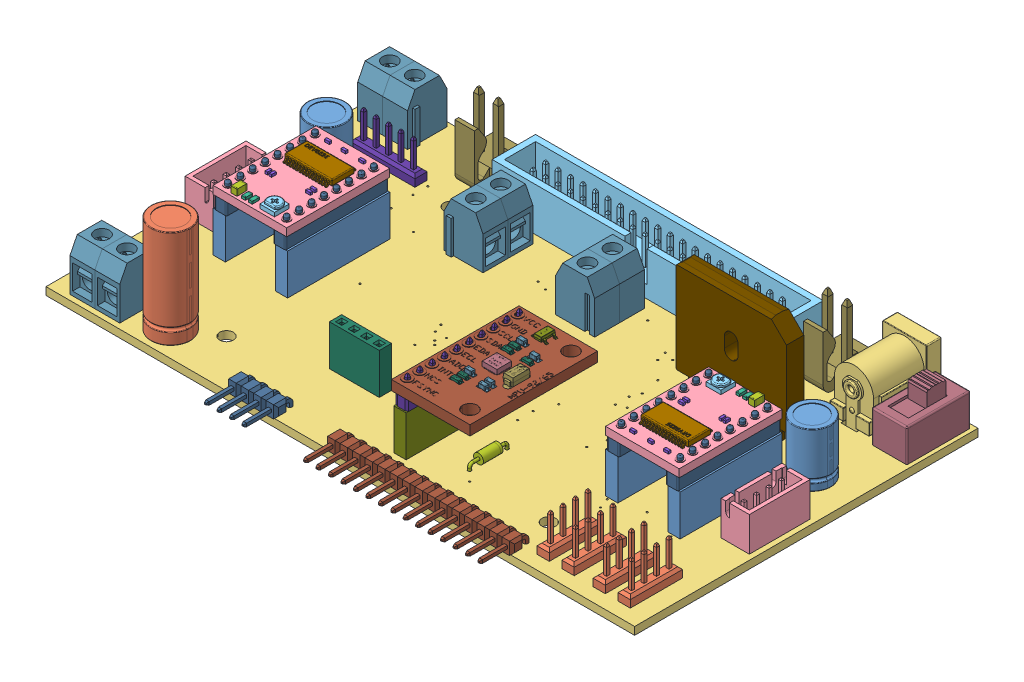
SolidWorks assembly RILey_PCB_V2, configuration Default. Lengths in mm.
Overall size (120 36.8 77.07).
114 component instances, 35 part files, 11 mates.
Components (placement in the parent):
- RILey-PCB_V2.0.step-1: RILey-PCB_V2.0.step [Default] at (-30.3949 55.9091 134.4073) x (1 0 0) z (0 1 0) size (120 77.07 36.8)
  - Packages.step-1: Packages.step [Default] at origin size (117.53 77.07 36.8)
    - CAPPRD250W50D655H1250.step-1: CAPPRD250W50D655H1250.step [Default] at (10.16 48.26 1.57) x (-1 0 0) z (0 0 1) size (7.62 7.6 12.92)
      - Model.step-1: Model.step [Default] at (1.2482 -0.0007 0.1237) size (7.62 7.6 12.92)
    - CAPPRD250W50D655H1250_1.step-1: CAPPRD250W50D655H1250_1.step [Default] at (110.49 44.45 1.57) size (7.62 7.6 12.92)
      - Model.step-1: Model.step [Default] at (1.2482 -0.0007 0.1237) size (7.62 7.6 12.92)
    - ELECTROLYTIC_CAPACITOR.step-1: ELECTROLYTIC_CAPACITOR.step [Default] at (20.32 5.08 1.57) size (8.02 8 21.92)
      - Model (1).step-1: Model (1).step [Default] at origin size (8.02 8 21.92)
    - 733980-62.step-1: 733980-62.step [Default] at (106.68 66.04 1.57) x (-1 0 0) z (0 0 1) size (9.55 14.2 15)
      - DS-210 v1.step-1: DS-210 v1.step [Default] at (-0.0014 -5.2814 0) x (-1 0 0) z (0 0 1) size (9.55 14.2 15)
    - B4B-XH-A_LF__SN_.step-1: B4B-XH-A_LF__SN_.step [Default] at (5.08 29.21 1.57) x (0 1 0) z (0 0 1) size (12.4 5.75 10.45)
      - JST XH 4 B4B-XH-A v1.step-1: JST XH 4 B4B-XH-A v1.step [Default] at (3.6633 0.5127 0.0202) x (1 0 0) z (0 -1 0) size (12.4 10.45 5.75)
    - B4B-XH-A_LF__SN_.step-2: B4B-XH-A_LF__SN_.step [Default] at (115.57 34.29 1.57) x (0 -1 0) z (0 0 1) size (12.4 5.75 10.45)
      - JST XH 4 B4B-XH-A v1.step-1: JST XH 4 B4B-XH-A v1.step [Default] at (3.6633 0.5127 0.0202) x (1 0 0) z (0 -1 0) size (12.4 10.45 5.75)
    - MC-254-40-00-ST-DIP.step-1: MC-254-40-00-ST-DIP.step [Default] at (61.214 63.5 1.57) size (58.67 8.85 11.85)
      - MC-254-40-00-ST-DIP v1.step-1: MC-254-40-00-ST-DIP v1.step [Default] at (-24.13 -1.27 0) size (58.67 8.85 11.85)
        - Model (2).step-1: Model (2).step [Default] at (0 2.54 0) size (58.67 8.85 11.85)
    - TSOP6_SOT457.step-1: TSOP6_SOT457.step [Default] at (17.78 48.26 0) x (-1 0 0) z (0 0 -1) size (3 3.1 1.1)
      - Model (3).step-1: Model (3).step [Default] at origin size (3 3.1 1.1)
    - ZENER-TH.step-1: ZENER-TH.step [Default] at (75.565 14.605 1.57) x (0 1 0) z (0 0 1) size (8.22 2 4.02)
      - Model (4).step-1: Model (4).step [Default] x (-1 0 0) z (0 0 1) size (8.22 2 4.02)
    - 1812L300MR.step-1: 1812L300MR.step [Default] at (71.0315 17.78 0) x (0 -1 0) z (0 0 -1) size (4.73 3.41 1)
      - Model (5).step-1: Model (5).step [Default] at origin size (4.73 3.41 1)
    - 2920L400_15MR.step-1: 2920L400_15MR.step [Default] at (109.22 52.07 0) x (1 0 0) z (0 0 -1) size (7.98 5.44 1.6)
      - Model (6).step-1: Model (6).step [Default] at origin size (7.98 5.44 1.6)
    - MA04-1W.step-1: MA04-1W.step [Default] at (42.0116 3.8608 1.57) x (-1 0 0) z (0 0 1) size (10.16 9.88 5.54)
      - Model (7).step-1: Model (7).step [Default] at (3.81 -0.002 0) x (-1 0 0) z (0 0 1) size (10.16 9.89 5.54)
    - MA15-1W.step-1: MA15-1W.step [Default] at (76.2 3.81 1.57) x (-1 0 0) z (0 0 1) size (38.1 9.89 5.54)
      - Model (8).step-1: Model (8).step [Default] at (17.78 0 0) x (-1 0 0) z (0 0 1) size (38.1 9.89 5.54)
    - KK41791-4020_2-PIN.step-1: KK41791-4020_2-PIN.step [Default] at (96.52 64.77 1.57) x (-1 0 0) z (0 0 1) size (7.77 10.01 17.02)
      - Molex-kk-396 v2.step-1: Molex-kk-396 v2.step [Default] at (0.0973 -2.0339 0.4801) x (1 0 0) z (0 -1 0) size (7.77 17.02 10.01)
        - 1.step-1: 1.step [Default] at (-0.1266 1.3496 -0.3443) size (7.77 17.02 10.01)
    - KK41791-4020_2-PIN_1.step-1: KK41791-4020_2-PIN_1.step [Default] at (25.4 64.77 1.57) x (-1 0 0) z (0 0 1) size (7.77 10.01 17.02)
      - Molex-kk-396 v2_1.step-1: Molex-kk-396 v2_1.step [Default] at (0.0973 -2.0339 0.4801) x (1 0 0) z (0 -1 0) size (7.77 17.02 10.01)
        - 1.step-1: 1.step [Default] at (-0.1266 1.3496 -0.3443) size (7.77 17.02 10.01)
    - 1000-SERIES(SPDT).step-1: 1000-SERIES(SPDT).step [Default] at (115.6208 62.7634 1.57) size (7.2 13 13.1)
      - SS-12M11G3 v2.step-1: SS-12M11G3 v2.step [Default] at origin size (7.2 13 13.1)
    - W237-102.step-1: W237-102.step [Default] at (7.5692 66.3194 1.57) size (10.66 8 14)
      - Schraubklemme_Blau_300V_16A_2P v1.step-1: Schraubklemme_Blau_300V_16A_2P v1.step [Default] at (-0.2451 0.529 2.8414) x (0 1 0) z (0 0 1) size (8 10.66 14)
        - Schraubklemme_Blau_300V_16A.step-1: Schraubklemme_Blau_300V_16A.step [Default] at (2.2082 -5.3326 -3) size (8 5.58 14)
        - Schraubklemme_Blau_300V_16A.step-2: Schraubklemme_Blau_300V_16A.step [Default] at (2.2082 -0.2526 -3) size (8 5.58 14)
    - W237-102_1.step-1: W237-102_1.step [Default] at (8.89 3.81 1.57) x (-1 0 0) z (0 0 1) size (10.66 8 14)
      - Schraubklemme_Blau_300V_16A_2P v1_1.step-1: Schraubklemme_Blau_300V_16A_2P v1_1.step [Default] at (-0.2451 0.529 2.8414) x (0 1 0) z (0 0 1) size (8 10.66 14)
        - Schraubklemme_Blau_300V_16A.step-1: Schraubklemme_Blau_300V_16A.step [Default] at (2.2082 -5.3326 -3) size (8 5.58 14)
        - Schraubklemme_Blau_300V_16A.step-2: Schraubklemme_Blau_300V_16A.step [Default] at (2.2082 -0.2526 -3) size (8 5.58 14)
    - W237-102_2.step-1: W237-102_2.step [Default] at (59.5884 52.07 1.57) x (0 1 0) z (0 0 1) size (10.66 8 14)
      - Schraubklemme_Blau_300V_16A_2P v1_2.step-1: Schraubklemme_Blau_300V_16A_2P v1_2.step [Default] at (-0.2451 0.529 2.8414) x (0 1 0) z (0 0 1) size (8 10.66 14)
        - Schraubklemme_Blau_300V_16A.step-1: Schraubklemme_Blau_300V_16A.step [Default] at (2.2082 -5.3326 -3) size (8 5.58 14)
        - Schraubklemme_Blau_300V_16A.step-2: Schraubklemme_Blau_300V_16A.step [Default] at (2.2082 -0.2526 -3) size (8 5.58 14)
    - W237-102_3.step-1: W237-102_3.step [Default] at (39.37 52.07 1.57) x (0 -1 0) z (0 0 1) size (10.66 8 14)
      - Schraubklemme_Blau_300V_16A_2P v1_3.step-1: Schraubklemme_Blau_300V_16A_2P v1_3.step [Default] at (-0.2451 0.529 2.8414) x (0 1 0) z (0 0 1) size (8 10.66 14)
        - Schraubklemme_Blau_300V_16A.step-1: Schraubklemme_Blau_300V_16A.step [Default] at (2.2082 -5.3326 -3) size (8 5.58 14)
        - Schraubklemme_Blau_300V_16A.step-2: Schraubklemme_Blau_300V_16A.step [Default] at (2.2082 -0.2526 -3) size (8 5.58 14)
    - FE04-1.step-1: FE04-1.step [Default] at (52.2732 15.6464 1.57) x (-1 0 0) z (0 0 1) size (10.16 2.5 11.3)
    - FE10-1.step-1: FE10-1.step [Default] at (66.04 19.0691 1.57) x (0 -1 0) z (0 0 1) size (25.9 2.5 11.3)
    - MA05-1_S.step-1: MA05-1_S.step [Default] at (13.97 55.88 1.57) x (-1 0 0) z (0 0 1) size (13.2 2.5 11)
    - DIODE-BRIDGE.step-1: DIODE-BRIDGE.step [Default] at (92.71 48.26 1.57) size (22.51 3.56 36.8)
    - FE08-1.step-1: FE08-1.step [Default] at (25.4 33.02 1.57) x (0 1 0) z (0 0 1) size (20.82 2.5 11.3)
    - FE08-1.step-2: FE08-1.step [Default] at (12.7 33.02 1.57) x (0 1 0) z (0 0 1) size (20.82 2.5 11.3)
    - FE08-1.step-3: FE08-1.step [Default] at (95.25 30.48 1.57) x (0 -1 0) z (0 0 1) size (20.82 2.5 11.3)
    - FE08-1.step-4: FE08-1.step [Default] at (107.95 30.48 1.57) x (0 -1 0) z (0 0 1) size (20.82 2.5 11.3)
    - MA04-1_S.step-1: MA04-1_S.step [Default] at (99.06 7.62 1.57) x (0 -1 0) z (0 0 1) size (10.66 2.5 11)
    - MA04-1_S.step-2: MA04-1_S.step [Default] at (104.14 7.62 1.57) x (0 -1 0) z (0 0 1) size (10.66 2.5 11)
    - MA04-1_S.step-3: MA04-1_S.step [Default] at (110.49 7.62 1.57) x (0 -1 0) z (0 0 1) size (10.66 2.5 11)
    - MA04-1_S.step-4: MA04-1_S.step [Default] at (115.57 7.62 1.57) x (0 -1 0) z (0 0 1) size (10.66 2.5 11)
  - Board.step-1: Board.step [Default] at origin size (120 70 1.57)
- DRV 8825 With Headers Assem-1: DRV 8825 With Headers Assem [Default] at (-1.0467 51.8574 109.5035) x (0 0 -1) z (0 1 0) size (21 15 10.9)
  - PCB-1: PCB [Default] at (8.1162 10.2982 16.4218) size (21 15 1.8)
  - SMD Pot-1: SMD Pot [Default] at (-0.2134 7.4613 18.0218) x (0 -1 0) z (0 0 1) size (3 3 1.3)
  - 0603 Resistor-1: 0603 Resistor [Default] at (-1.0068 10.8561 18.0218) size (1.5 0.8 0.5)
  - 0603 Resistor-2: 0603 Resistor [Default] at (-1.0286 12.2306 18.0218) size (1.5 0.8 0.5)
  - 0805 Capacitor-1: 0805 Capacitor [Default] at (-0.8941 14.0417 18.0218) size (2 1.25 1.25)
  - 0402 Resistor-1: 0402 Resistor [Default] at (16.8896 6.6863 18.0218) x (0 -1 0) z (0 0 1) size (1 0.68 0.66)
  - 0402 Resistor-2: 0402 Resistor [Default] at (16.8896 10.308 18.0218) x (0 -1 0) z (0 0 1) size (1 0.68 0.66)
  - 0402 Resistor-3: 0402 Resistor [Default] at (16.8896 13.6408 18.0218) x (0 -1 0) z (0 0 1) size (1 0.68 0.66)
  - 0402 Resistor-4: 0402 Resistor [Default] at (6.8882 6.5987 18.0218) x (0 -1 0) z (0 0 1) size (1 0.68 0.66)
  - 0402 Resistor-5: 0402 Resistor [Default] at (5.9719 6.5987 18.0218) x (0 -1 0) z (0 0 1) size (1 0.68 0.66)
  - 0402 Resistor-6: 0402 Resistor [Default] at (5.456 14.3274 18.0218) size (1 0.68 0.66)
  - 0402 Resistor-7: 0402 Resistor [Default] at (5.456 13.4855 18.0218) size (1 0.68 0.66)
  - DRV8825 IC-1: DRV8825 IC [Default] at (11.7347 10.2312 18.0218) x (0 -1 0) z (0 0 1) size (9.6 6.2 1.2)
  - 8 pin Header-1: 8 pin Header [Default] at (8.1162 16.2982 13.9218) size (21 2.5 10.5)
  - 8 pin Header-2: 8 pin Header [Default] at (8.1162 4.2982 13.9218) size (21 2.5 10.5)
- DRV 8825 With Headers Assem-2: DRV 8825 With Headers Assem [Default] at (60.9069 51.8574 95.811) x (0 0 1) z (0 1 0) size (21 15 10.9)
  - PCB-1: PCB [Default] at (8.1162 10.2982 16.4218) size (21 15 1.8)
  - SMD Pot-1: SMD Pot [Default] at (-0.2134 7.4613 18.0218) x (0 -1 0) z (0 0 1) size (3 3 1.3)
  - 0603 Resistor-1: 0603 Resistor [Default] at (-1.0068 10.8561 18.0218) size (1.5 0.8 0.5)
  - 0603 Resistor-2: 0603 Resistor [Default] at (-1.0286 12.2306 18.0218) size (1.5 0.8 0.5)
  - 0805 Capacitor-1: 0805 Capacitor [Default] at (-0.8941 14.0417 18.0218) size (2 1.25 1.25)
  - 0402 Resistor-1: 0402 Resistor [Default] at (16.8896 6.6863 18.0218) x (0 -1 0) z (0 0 1) size (1 0.68 0.66)
  - 0402 Resistor-2: 0402 Resistor [Default] at (16.8896 10.308 18.0218) x (0 -1 0) z (0 0 1) size (1 0.68 0.66)
  - 0402 Resistor-3: 0402 Resistor [Default] at (16.8896 13.6408 18.0218) x (0 -1 0) z (0 0 1) size (1 0.68 0.66)
  - 0402 Resistor-4: 0402 Resistor [Default] at (6.8882 6.5987 18.0218) x (0 -1 0) z (0 0 1) size (1 0.68 0.66)
  - 0402 Resistor-5: 0402 Resistor [Default] at (5.9719 6.5987 18.0218) x (0 -1 0) z (0 0 1) size (1 0.68 0.66)
  - 0402 Resistor-6: 0402 Resistor [Default] at (5.456 14.3274 18.0218) size (1 0.68 0.66)
  - 0402 Resistor-7: 0402 Resistor [Default] at (5.456 13.4855 18.0218) size (1 0.68 0.66)
  - DRV8825 IC-1: DRV8825 IC [Default] at (11.7347 10.2312 18.0218) x (0 -1 0) z (0 0 1) size (9.6 6.2 1.2)
  - 8 pin Header-1: 8 pin Header [Default] at (8.1162 16.2982 13.9218) size (21 2.5 10.5)
  - 8 pin Header-2: 8 pin Header [Default] at (8.1162 4.2982 13.9218) size (21 2.5 10.5)
- MPU9250.STEP-1: MPU9250.STEP [Default] at (68.1451 69.3424 118.518) x (0 0 1) z (-1 0 0) size (26 3.91 16)
  - PCB.STEP-1: PCB.STEP [Default] at (-2.9998 1.0768 26) size (26 2.2 16)
  - C2.STEP-1: C2.STEP [Default] at (-2.4989 2.0768 21) x (0 0 -1) z (1 0 0) size (2 1.81 5.01)
  - MP92.STEP-1: MP92.STEP [Default] at (-2.9998 1.0968 25.5) x (0 0 -1) z (1 0 0) size (3.29 1.01 3.29)
  - C1_Predeterminado_Como mecanizada_.STEP-1: C1_Predeterminado_Como mecanizada_.STEP [Default] at (2.1384 1.0968 23.0905) x (0 0 1) z (-1 0 0) size (2.2 0.83 0.9)
  - C1_Predeterminado_Como mecanizada_.STEP-2: C1_Predeterminado_Como mecanizada_.STEP [Default] at (0.9102 1.0968 27.1044) x (0 0 1) z (-1 0 0) size (2.2 0.83 0.9)
  - C1_Predeterminado_Como mecanizada_.STEP-3: C1_Predeterminado_Como mecanizada_.STEP [Default] at (0.9102 1.0968 23.0905) x (0 0 1) z (-1 0 0) size (2.2 0.83 0.9)
  - C1_Predeterminado_Como mecanizada_.STEP-4: C1_Predeterminado_Como mecanizada_.STEP [Default] at (-8.3098 1.0968 23.0905) x (0 0 1) z (-1 0 0) size (2.2 0.83 0.9)
  - C1_Predeterminado_Como mecanizada_.STEP-5: C1_Predeterminado_Como mecanizada_.STEP [Default] at (-9.7098 1.0968 27.1044) x (0 0 1) z (-1 0 0) size (2.2 0.83 0.9)
  - R1.STEP-1: R1.STEP [Default] at (3.5484 1.1168 27.2144) x (0 0 -1) z (1 0 0) size (2.2 0.47 0.9)
  - R1.STEP-2: R1.STEP [Default] at (2.1484 1.1168 27.2144) x (0 0 -1) z (1 0 0) size (2.2 0.47 0.9)
  - R1.STEP-3: R1.STEP [Default] at (-6.8998 1.1168 23.2005) x (0 0 -1) z (1 0 0) size (2.2 0.47 0.9)
  - R1.STEP-4: R1.STEP [Default] at (-8.2998 1.1168 27.2144) x (0 0 -1) z (1 0 0) size (2.2 0.47 0.9)
  - R1.STEP-5: R1.STEP [Default] at (-6.8998 1.1168 27.2144) x (0 0 -1) z (1 0 0) size (2.2 0.47 0.9)
  - V1.STEP-1: V1.STEP [Default] at (-13.0785 1.5868 25.9) size (2.9 0.96 3.2)
- PinHeader10row-1: PinHeader10row [Default] at (36.9151 68.3191 125.4982) x (0 0 1) z (1 0 0) size (25.4 11.54 2.54)
Mates (geometry in assembly coordinates):
- ProfileCenter1: profile center = 1.85 mm anti-aligned: plane of PinHeader10row-1 through (36.9151 59.7791 125.4982) normal (0 -1 0); plane of RILey-PCB_V2.0.step-1/Packages.step-1/FE10-1.step-1 through (35.6451 61.6291 126.7682) normal (0 1 0)
- Concentric1: concentric: cylinder of RILey-PCB_V2.0.step-1/Board.step-1 through (35.6451 -144.0909 126.7682) axis (0 1 0) radius 0.5776; cylinder of MPU9250.STEP-1/PCB.STEP-1 through (35.6451 68.4191 126.7682) axis (0 1 0) radius 0.5
- Parallel3: parallel: plane of RILey-PCB_V2.0.step-1/Packages.step-1/FE10-1.step-1 through (34.3951 61.6291 115.3382) normal (-1 0 0); plane of MPU9250.STEP-1/PCB.STEP-1 through (34.1451 68.4191 115.5182) normal (-1 0 0)
- Parallel4: parallel: plane of RILey-PCB_V2.0.step-1/Packages.step-1/FE10-1.step-1 through (35.6451 61.6291 128.2882) normal (0 0 1); plane of MPU9250.STEP-1/PCB.STEP-1 through (42.1451 68.4191 128.5182) normal (0 0 1)
- Coincident3: coincident anti-aligned: plane of MPU9250.STEP-1/PCB.STEP-1 through (42.1451 68.3191 115.5182) normal (0 -1 0); plane of PinHeader10row-1 through (36.9151 68.3191 125.4982) normal (0 1 0)
- Width1: width: plane of DRV 8825 With Headers Assem-1/PCB-1 through (-3.8449 69.8791 111.8873) normal (1 0 0); plane of DRV 8825 With Headers Assem-1/PCB-1 through (-18.8449 69.8791 111.8873) normal (-1 0 0); plane of RILey-PCB_V2.0.step-1/Packages.step-1/FE08-1.step-2 through (-18.9449 61.6291 101.3873) normal (-1 0 0); plane of RILey-PCB_V2.0.step-1/Packages.step-1/FE08-1.step-1 through (-3.7449 61.6291 101.3873) normal (1 0 0)
- Width2: width: plane of DRV 8825 With Headers Assem-1/PCB-1 through (-18.8449 69.8791 111.8873) normal (0 0 1); plane of DRV 8825 With Headers Assem-1/PCB-1 through (-18.8449 69.8791 90.8873) normal (0 0 -1); plane of RILey-PCB_V2.0.step-1/Packages.step-1/FE08-1.step-1 through (-4.9949 61.6291 90.9773) normal (0 0 -1); plane of RILey-PCB_V2.0.step-1/Packages.step-1/FE08-1.step-1 through (-4.9949 61.6291 111.7973) normal (0 0 1)
- Coincident4: coincident anti-aligned: plane of RILey-PCB_V2.0.step-1/Packages.step-1/FE08-1.step-1 through (-4.9949 65.7791 101.3873) normal (0 1 0); plane of DRV 8825 With Headers Assem-1/8 pin Header-2 through (-5.3449 65.7791 101.3873) normal (0 -1 0)
- Width3: width: plane of DRV 8825 With Headers Assem-2/PCB-1 through (78.7051 69.8791 114.4273) normal (0 0 1); plane of DRV 8825 With Headers Assem-2/PCB-1 through (78.7051 69.8791 93.4273) normal (0 0 -1); plane of RILey-PCB_V2.0.step-1/Packages.step-1/FE08-1.step-3 through (64.8551 61.6291 114.3373) normal (0 0 1); plane of RILey-PCB_V2.0.step-1/Packages.step-1/FE08-1.step-3 through (64.8551 61.6291 93.5173) normal (0 0 -1)
- Width4: width: plane of DRV 8825 With Headers Assem-2/PCB-1 through (78.7051 69.8791 93.4273) normal (1 0 0); plane of DRV 8825 With Headers Assem-2/PCB-1 through (63.7051 69.8791 93.4273) normal (-1 0 0); plane of RILey-PCB_V2.0.step-1/Packages.step-1/FE08-1.step-3 through (63.6051 61.6291 103.9273) normal (-1 0 0); plane of RILey-PCB_V2.0.step-1/Packages.step-1/FE08-1.step-4 through (78.8051 61.6291 103.9273) normal (1 0 0)
- Coincident5: coincident anti-aligned: plane of RILey-PCB_V2.0.step-1/Packages.step-1/FE08-1.step-4 through (77.5551 65.7791 103.9273) normal (0 1 0); plane of DRV 8825 With Headers Assem-2/8 pin Header-1 through (77.2051 65.7791 103.9273) normal (0 -1 0)
